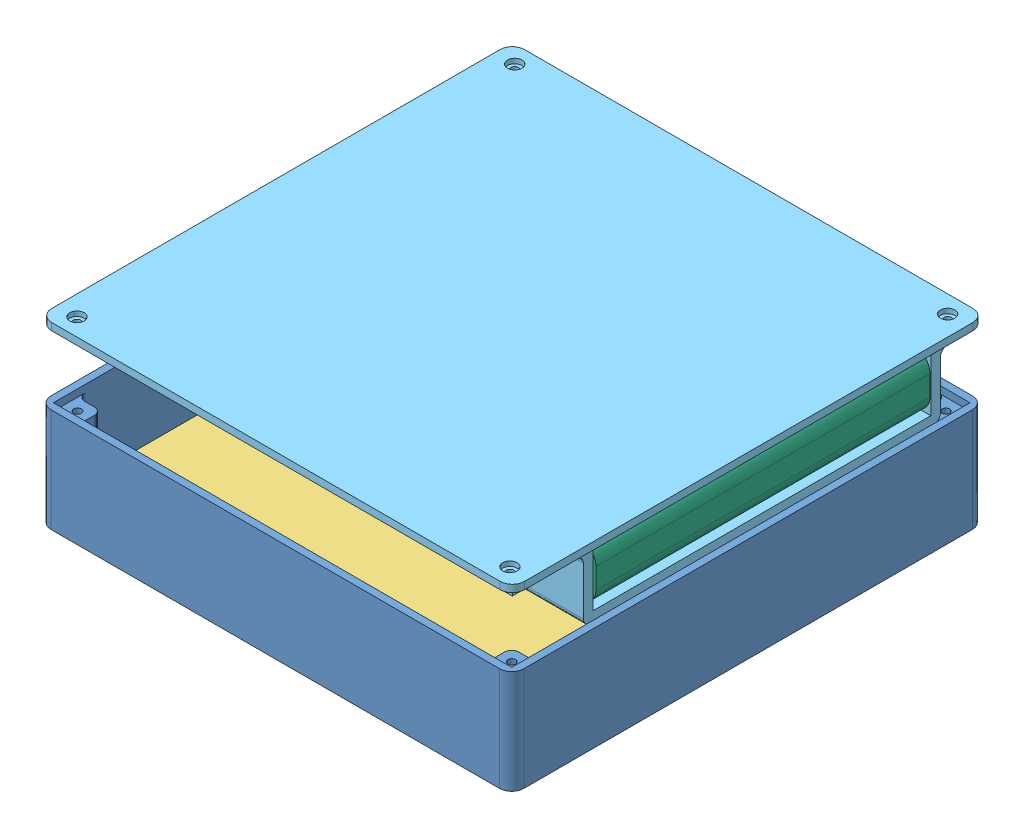
SolidWorks assembly PCB box wide assembly, configuration Default. Lengths in mm.
Overall size (196.25 74.47 196).
11 component instances, 6 part files, 20 mates.
Components (placement in the parent):
- PCB Box wide-1: PCB Box wide [Default] at origin size (196 43 196)
- Load cell-1: Load cell [Default] at (-73.9 4 -2.7) x (0 0 -1) z (1 0 0) size (32 2 25)
- PCB board-1: PCB board [Default] at (-10 5 54.6) size (167.6 2 58.4)
- Load cell-2: Load cell [Default] at (-36.9 4 -2.7) x (0 0 -1) z (1 0 0) size (32 2 25)
- Load cell-3: Load cell [Default] at (0.1 4 -2.7) x (0 0 -1) z (1 0 0) size (32 2 25)
- Load cell-4: Load cell [Default] at (37.1 4 -2.7) x (0 0 -1) z (1 0 0) size (32 2 25)
- arduino uno-2: arduino uno [Default] at (-29.2 11.65 -23.96) size (53.34 15.25 74.93)
- arduino uno-3: arduino uno [Default] at (30.8 11.65 -23.96) size (53.34 15.25 74.93)
- PCB lid wide-1: PCB lid wide [Default] at (0.25 71.4732 0) x (1 0 0) z (0 0 -1) size (196 32 196)
- Load cell-5: Load cell [Default] at (74.1 4 -2.7) x (0 0 -1) z (1 0 0) size (32 2 25)
- CPS1-Step.step-1: CPS1-Step.step [Default] at (72.0185 42.9044 -78.75) x (-1 0 0) z (0 1 0) size (60.7 139.8 21.57)
Mates (geometry in assembly coordinates):
- Coincident1: coincident anti-aligned: circle of PCB Box wide-1; plane of PCB board-1 through (-10 5 54.6) normal (0 -1 0)
- Coincident2: coincident anti-aligned: cylinder of PCB Box wide-1 through (-90 5 29.2) axis (0 -1 0) radius 1.6; circle of PCB board-1
- Coincident3: coincident anti-aligned: cylinder of PCB Box wide-1 through (-90 5 80) axis (0 -1 0) radius 1.6; circle of PCB board-1
- Coincident4: coincident anti-aligned: plane of PCB Box wide-1 through (-65 4 10) normal (0 1 0); plane of Load cell-1 through (-73.9 4 -2.7) normal (0 -1 0)
- Coincident5: coincident anti-aligned: cylinder of PCB Box wide-1 through (-65 4 10) axis (0 -1 0) radius 1.6; circle of Load cell-1
- Coincident6: coincident anti-aligned: cylinder of PCB Box wide-1 through (-65 4 -15.4) axis (0 -1 0) radius 1.6; circle of Load cell-1
- Coincident7: coincident: plane of PCB Box wide-1 through (-80 10 -39.2) normal (0 1 0); plane of arduino uno-1 through (1.04 5 -85.62) normal (0 -1 0)
- Concentric1: concentric: cylinder of PCB Box wide-1 through (-80 10 -39.2) axis (0 -1 0) radius 1.6; cylinder of arduino uno-1 through (-65 5 -50.06) axis (0 1 0) radius 1.5875
- Concentric2: concentric anti-aligned: cylinder of PCB Box wide-1 through (-31.74 10 -37.93) axis (0 -1 0) radius 1.6; cylinder of arduino uno-1 through (-14.2 5 -34.82) axis (0 1 0) radius 1.5875
- Concentric3: concentric anti-aligned: cylinder of PCB Box wide-1 through (-64.76 10 -90) axis (0 -1 0) radius 1.6; cylinder of arduino uno-2 through (-64.76 10 -90) axis (0 1 0) radius 1.5875
- Coincident9: coincident anti-aligned: plane of PCB Box wide-1 through (-80 10 -39.2) normal (0 1 0); plane of arduino uno-2 through (-29.2 10 -23.96) normal (0 -1 0)
- Concentric4: concentric anti-aligned: cylinder of PCB Box wide-1 through (-31.74 10 -37.93) axis (0 -1 0) radius 1.6; cylinder of arduino uno-2 through (-31.74 10 -37.93) axis (0 1 0) radius 1.5875
- Coincident10: coincident anti-aligned: plane of Power bank-1 through (66 205.9588 -33.5) normal (0 1 0); plane of PCB lid wide-1 through (0.25 65.4732 0) normal (0 -1 0)
- Coincident11: coincident anti-aligned: plane of Power bank-1 through (97 205.9588 -78.75) normal (0 0 -1); plane of PCB lid wide-1 through (95 43.4732 -78.75) normal (0 0 1)
- Coincident12: coincident anti-aligned: plane of Power bank-1 through (35 205.9588 11.75) normal (-1 0 0); plane of PCB lid wide-1 through (35 43.4732 -78.75) normal (1 0 0)
- Coincident13: coincident anti-aligned: plane of PCB Box wide-1 through (95 40 95) normal (-1 0 0); plane of PCB lid wide-1 through (95 65.4732 94.75) normal (1 0 0)
- Coincident15: coincident aligned: plane of PCB Box wide-1 through (-95 40 98) normal (0 0 1); plane of PCB lid wide-1 through (-97.75 68.4732 98) normal (0 0 1)
- Coincident16: coincident anti-aligned: plane of PCB lid wide-1 through (0.25 43.4732 0) normal (0 1 0); plane of CPS1-Step.step-1 through (64.5 43.4732 -9.5) normal (0 -1 0)
- Coincident17: coincident anti-aligned: plane of PCB lid wide-1 through (35 43.4732 -78.75) normal (1 0 0); plane of CPS1-Step.step-1 through (35 43.4732 59.75) normal (-1 0 0)
- Coincident18: coincident anti-aligned: plane of PCB lid wide-1 through (95 43.4732 -78.75) normal (0 0 1); plane of CPS1-Step.step-1 through (35 43.4732 -78.75) normal (0 0 -1)
